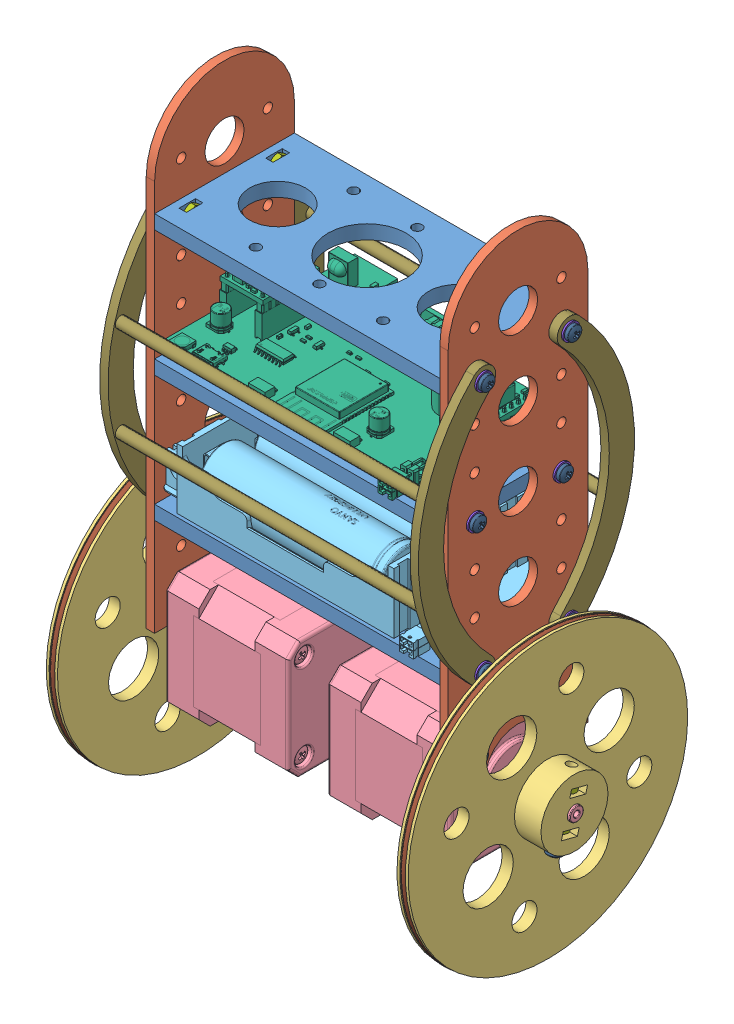
SolidWorks assembly RobotBalancin, configuration Predeterminado. Lengths in mm.
Overall size (150 233.71 126.43).
103 component instances, 13 part files, 199 mates.
Components (placement in the parent):
- RobotMiddle-1: RobotMiddle [Default] at (49.6239 154.592 64.1485) size (102 5 50)
- RobotLateral-1: RobotLateral [Default] at (100.3895 203.5472 64.288) size (3 165 50)
- RobotLateral-2: RobotLateral [Default] at (-4.6105 203.5472 64.288) size (3 165 50)
- RobotWheel-1: RobotWheel [Default] at (-11.3593 114.092 64.3829) x (0 -0.315254 -0.949007) z (-1 0 0) size (100 100 13.5)
- RobotWheel-2: RobotWheel [Default] at (110.074 114.092 64.3829) x (0 -0.248427 -0.968651) z (1 0 0) size (100 100 13.5)
- NEMA17-1: NEMA17 [Predeterminado] at (42.3895 109.4749 74.7784) x (0 0 1) z (-1 0 0) size (42.3 42.3 68)
- NEMA17-2: NEMA17 [Predeterminado] at (56.3895 109.4749 53.9874) x (0 0 -1) z (1 0 0) size (42.3 42.3 68)
- RobotMiddle-2: RobotMiddle [Default] at (49.6239 199.592 64.1485) size (102 5 50)
- RobotMiddle-3: RobotMiddle [Default] at (49.6239 244.592 64.1485) size (102 5 50)
- PowerBoard-4: PowerBoard [Predeterminado] at (99.6419 165.2035 39.6765) x (-1 0 0) z (0 1 0) size (100 62.58 25.48)
- ControlBoard-1: ControlBoard [Predeterminado] at (99.6279 210.2035 39.6365) x (-1 0 0) z (0 1 0) size (100 63.99 44.22)
- hex nut style 1 gradeab_iso-1: hex nut style 1 gradeab_iso [ISO - 4032 - M2.5 - D - N] at (97.0495 157.092 48.8829) x (0 0 -1) z (1 0 0) size (5 5.77 2)
- hex nut style 1 gradeab_iso-2: hex nut style 1 gradeab_iso [ISO - 4032 - M2.5 - D - N] at (1.6495 157.092 48.8829) x (0 0 1) z (-1 0 0) size (5 5.77 2)
- hex nut style 1 gradeab_iso-3: hex nut style 1 gradeab_iso [ISO - 4032 - M2.5 - D - N] at (1.6495 157.092 79.8829) x (0 0 1) z (-1 0 0) size (5 5.77 2)
- hex nut style 1 gradeab_iso-4: hex nut style 1 gradeab_iso [ISO - 4032 - M2.5 - D - N] at (97.0495 157.092 79.8829) x (0 0 -1) z (1 0 0) size (5 5.77 2)
- hex nut style 1 gradeab_iso-5: hex nut style 1 gradeab_iso [ISO - 4032 - M2.5 - D - N] at (97.0495 202.092 79.8829) x (0 0 -1) z (1 0 0) size (5 5.77 2)
- hex nut style 1 gradeab_iso-6: hex nut style 1 gradeab_iso [ISO - 4032 - M2.5 - D - N] at (97.0495 202.092 48.8829) x (0 0 -1) z (1 0 0) size (5 5.77 2)
- hex nut style 1 gradeab_iso-7: hex nut style 1 gradeab_iso [ISO - 4032 - M2.5 - D - N] at (1.6495 202.092 79.8829) x (0 0 1) z (-1 0 0) size (5 5.77 2)
- hex nut style 1 gradeab_iso-8: hex nut style 1 gradeab_iso [ISO - 4032 - M2.5 - D - N] at (1.6495 202.092 48.8829) x (0 0 1) z (-1 0 0) size (5 5.77 2)
- plain washer 10673 type snl_iso-1: plain washer 10673 type snl_iso [ISO 10673-2.75-S] at (49.6239 154.592 46.6485) x (0 -1 0) z (0 0 1) size (0.6 6 6)
- plain washer 10673 type snl_iso-2: plain washer 10673 type snl_iso [ISO 10673-2.75-S] at (72.3739 154.592 81.6485) x (0 -1 0) z (0 0 1) size (0.6 6 6)
- plain washer 10673 type snl_iso-3: plain washer 10673 type snl_iso [ISO 10673-2.75-S] at (26.8739 154.592 81.6485) x (0 -1 0) z (0 0 1) size (0.6 6 6)
- plain washer 10673 type snl_iso-6: plain washer 10673 type snl_iso [ISO 10673-2.75-S] at (-4.6105 202.092 79.8829) x (-1 0 0) z (0 0.924225 0.381849) size (0.6 6 6)
- plain washer 10673 type snl_iso-7: plain washer 10673 type snl_iso [ISO 10673-2.75-S] at (-4.6105 202.092 48.8829) x (-1 0 0) z (0 0.924225 0.381849) size (0.6 6 6)
- plain washer 10673 type snl_iso-12: plain washer 10673 type snl_iso [ISO 10673-2.75-S] at (103.3895 202.092 48.8829) size (0.6 6 6)
- plain washer 10673 type snl_iso-13: plain washer 10673 type snl_iso [ISO 10673-2.75-S] at (103.3895 202.092 79.8829) size (0.6 6 6)
- plain washer 10673 type snl_iso-17: plain washer 10673 type snl_iso [ISO 10673-2.75-S] at (72.3739 199.592 46.6485) x (0 -1 0) z (0 0 1) size (0.6 6 6)
- plain washer 10673 type snl_iso-18: plain washer 10673 type snl_iso [ISO 10673-2.75-S] at (26.8739 199.592 46.6485) x (0 -1 0) z (0 0 1) size (0.6 6 6)
- plain washer 10673 type snl_iso-19: plain washer 10673 type snl_iso [ISO 10673-2.75-S] at (49.6239 159.592 46.6485) x (0 1 0) z (0 0 1) size (0.6 6 6)
- plain washer 10673 type snl_iso-20: plain washer 10673 type snl_iso [ISO 10673-2.75-S] at (26.8739 159.592 81.6485) x (0 1 0) z (0 0 1) size (0.6 6 6)
- plain washer 10673 type snl_iso-21: plain washer 10673 type snl_iso [ISO 10673-2.75-S] at (72.3739 159.592 81.6485) x (0 1 0) z (0 0 1) size (0.6 6 6)
- plain washer 10673 type snl_iso-22: plain washer 10673 type snl_iso [ISO 10673-2.75-S] at (72.3739 204.592 46.6485) x (0 1 0) z (0 0 1) size (0.6 6 6)
- plain washer 10673 type snl_iso-23: plain washer 10673 type snl_iso [ISO 10673-2.75-S] at (26.8739 204.592 46.6485) x (0 1 0) z (0 0 1) size (0.6 6 6)
- hex nut style 1 gradeab_iso-9: hex nut style 1 gradeab_iso [ISO - 4032 - M2.5 - D - N] at (49.6239 162.192 46.6485) x (1 0 0) z (0 1 0) size (5 5.77 2)
- hex nut style 1 gradeab_iso-10: hex nut style 1 gradeab_iso [ISO - 4032 - M2.5 - D - N] at (72.3739 162.192 81.6485) x (1 0 0) z (0 1 0) size (5 5.77 2)
- hex nut style 1 gradeab_iso-11: hex nut style 1 gradeab_iso [ISO - 4032 - M2.5 - D - N] at (26.8739 162.192 81.6485) x (1 0 0) z (0 1 0) size (5 5.77 2)
- hex nut style 1 gradeab_iso-12: hex nut style 1 gradeab_iso [ISO - 4032 - M2.5 - D - N] at (26.8739 207.192 46.6485) x (1 0 0) z (0 1 0) size (5 5.77 2)
- hex nut style 1 gradeab_iso-15: hex nut style 1 gradeab_iso [ISO - 4032 - M2.5 - D - N] at (26.8739 209.192 46.6485) x (1 0 0) z (0 1 0) size (5 5.77 2)
- hex nut style 1 gradeab_iso-16: hex nut style 1 gradeab_iso [ISO - 4032 - M2.5 - D - N] at (26.8739 164.192 81.6485) x (1 0 0) z (0 1 0) size (5 5.77 2)
- hex nut style 1 gradeab_iso-17: hex nut style 1 gradeab_iso [ISO - 4032 - M2.5 - D - N] at (49.6239 164.192 46.6485) x (1 0 0) z (0 1 0) size (5 5.77 2)
- hex nut style 1 gradeab_iso-18: hex nut style 1 gradeab_iso [ISO - 4032 - M2.5 - D - N] at (72.3739 164.192 81.6485) x (1 0 0) z (0 1 0) size (5 5.77 2)
- hex nut style 1 gradeab_iso-20: hex nut style 1 gradeab_iso [ISO - 4032 - M2.5 - D - N] at (72.3739 207.192 46.6485) x (1 0 0) z (0 1 0) size (5 5.77 2)
- hex nut style 1 gradeab_iso-21: hex nut style 1 gradeab_iso [ISO - 4032 - M2.5 - D - N] at (72.3739 209.192 46.6485) x (1 0 0) z (0 1 0) size (5 5.77 2)
- plain washer 10673 type snl_iso-24: plain washer 10673 type snl_iso [ISO 10673-2.75-S] at (72.3739 209.192 46.6485) x (0 1 0) z (0 0 1) size (0.6 6 6)
- plain washer 10673 type snl_iso-25: plain washer 10673 type snl_iso [ISO 10673-2.75-S] at (26.8739 209.192 46.6485) x (0 1 0) z (0 0 1) size (0.6 6 6)
- plain washer 10673 type snl_iso-26: plain washer 10673 type snl_iso [ISO 10673-2.75-S] at (26.8739 164.192 81.6485) x (0 1 0) z (0 0 1) size (0.6 6 6)
- plain washer 10673 type snl_iso-27: plain washer 10673 type snl_iso [ISO 10673-2.75-S] at (72.3739 164.192 81.6485) x (0 1 0) z (0 0 1) size (0.6 6 6)
- plain washer 10673 type snl_iso-28: plain washer 10673 type snl_iso [ISO 10673-2.75-S] at (49.6239 164.192 46.6485) x (0 1 0) z (0 0 1) size (0.6 6 6)
- plain washer 10673 type snl_iso-30: plain washer 10673 type snl_iso [ISO 10673-2.75-S] at (72.3739 210.2035 46.6485) x (0 1 0) z (0 0 1) size (0.6 6 6)
- plain washer 10673 type snl_iso-31: plain washer 10673 type snl_iso [ISO 10673-2.75-S] at (26.8739 210.2035 46.6485) x (0 1 0) z (0 0 1) size (0.6 6 6)
- countersunk flat head cross recess screw_iso-1: countersunk flat head cross recess screw_iso [ISO 7046-1 - M2.5 x 16 - Z - 16N] at (49.6155 166.8314 46.6547) x (0 -1 0) z (0.014601 0 0.999893) size (16 4.7 4.7)
- countersunk flat head cross recess screw_iso-2: countersunk flat head cross recess screw_iso [ISO 7046-1 - M2.5 x 16 - Z - 16N] at (72.3655 166.8314 81.6547) x (0 -1 0) z (-0.020315 0 0.999794) size (16 4.7 4.7)
- countersunk flat head cross recess screw_iso-3: countersunk flat head cross recess screw_iso [ISO 7046-1 - M2.5 x 16 - Z - 16N] at (26.8655 166.8314 81.6547) x (0 -1 0) z (-0.013089 0 0.999914) size (16 4.7 4.7)
- pan head cross recess screw_iso-1: pan head cross recess screw_iso [ISO 7045 - M2.5 x 16 - Z - 16N] at (72.3739 212.9035 46.6485) x (0 -1 0) z (0 0 1) size (18.05 5 5)
- pan head cross recess screw_iso-2: pan head cross recess screw_iso [ISO 7045 - M2.5 x 16 - Z - 16N] at (26.8739 212.9035 46.6485) x (0 -1 0) z (0 0 1) size (18.05 5 5)
- pan head cross recess screw_iso-5: pan head cross recess screw_iso [ISO 7045 - M2.5 x 8 - Z - 8N] at (106.0895 202.092 48.8829) x (-1 0 0) z (0 0.924225 0.381849) size (10.05 5 5)
- pan head cross recess screw_iso-6: pan head cross recess screw_iso [ISO 7045 - M2.5 x 8 - Z - 8N] at (106.0895 202.092 79.8829) x (-1 0 0) z (0 0.924225 0.381849) size (10.05 5 5)
- pan head cross recess screw_iso-11: pan head cross recess screw_iso [ISO 7045 - M2.5 x 8 - Z - 8N] at (-7.3105 202.092 79.8829) size (10.05 5 5)
- pan head cross recess screw_iso-12: pan head cross recess screw_iso [ISO 7045 - M2.5 x 8 - Z - 8N] at (-7.3105 202.092 48.8829) size (10.05 5 5)
- plain washer 10673 type snl_iso-32: plain washer 10673 type snl_iso [ISO 10673-2.75-S] at (103.3895 129.592 48.8829) size (0.6 6 6)
- plain washer 10673 type snl_iso-33: plain washer 10673 type snl_iso [ISO 10673-2.75-S] at (103.3895 129.592 79.8829) size (0.6 6 6)
- plain washer 10673 type snl_iso-34: plain washer 10673 type snl_iso [ISO 10673-2.75-S] at (-4.6105 129.592 48.8829) x (-1 0 0) z (0 0.924225 0.381849) size (0.6 6 6)
- plain washer 10673 type snl_iso-35: plain washer 10673 type snl_iso [ISO 10673-2.75-S] at (-4.6105 129.592 79.8829) x (-1 0 0) z (0 0.924225 0.381849) size (0.6 6 6)
- pan head cross recess screw_iso-17: pan head cross recess screw_iso [ISO 7045 - M3 x 8 - Z - 8N] at (-7.6105 129.592 48.8829) size (10.35 5.6 5.6)
- pan head cross recess screw_iso-18: pan head cross recess screw_iso [ISO 7045 - M3 x 8 - Z - 8N] at (-7.6105 129.592 79.8829) size (10.35 5.6 5.6)
- pan head cross recess screw_iso-19: pan head cross recess screw_iso [ISO 7045 - M3 x 8 - Z - 8N] at (106.3895 129.592 48.8829) x (-1 0 0) z (0 0.924225 0.381849) size (10.35 5.6 5.6)
- pan head cross recess screw_iso-20: pan head cross recess screw_iso [ISO 7045 - M3 x 8 - Z - 8N] at (106.3895 129.592 79.8829) x (-1 0 0) z (0 0.924225 0.381849) size (10.35 5.6 5.6)
- hex nut style 1 gradeab_iso-22: hex nut style 1 gradeab_iso [ISO - 4032 - M2.5 - D - N] at (119.574 120.582 62.7184) x (1 0 0) z (0 0.968651 -0.248427) size (5 5.77 2)
- hex nut style 1 gradeab_iso-23: hex nut style 1 gradeab_iso [ISO - 4032 - M2.5 - D - N] at (119.574 107.6021 66.0474) x (1 0 0) z (0 -0.968651 0.248427) size (5 5.77 2)
- hex nut style 1 gradeab_iso-24: hex nut style 1 gradeab_iso [ISO - 4032 - M2.5 - D - N] at (-20.8593 120.4504 62.2707) x (1 0 0) z (0 0.949007 -0.315254) size (5 5.77 2)
- hex nut style 1 gradeab_iso-25: hex nut style 1 gradeab_iso [ISO - 4032 - M2.5 - D - N] at (-20.8593 107.7337 66.4951) x (1 0 0) z (0 -0.949007 0.315254) size (5 5.77 2)
- pan head cross recess screw_iso-23: pan head cross recess screw_iso [ISO 7045 - M2.5 x 20 - Z - 20N] at (-20.8593 127.473 59.9378) x (0 -0.949007 0.315254) z (-0.315254 0.299178 0.900615) size (22.05 5 5)
- pan head cross recess screw_iso-24: pan head cross recess screw_iso [ISO 7045 - M2.5 x 20 - Z - 20N] at (119.574 100.4341 67.8857) x (0 0.968651 -0.248427) z (0.248427 0.240639 0.938284) size (22.05 5 5)
- o-rings series g_iso-1: o-rings series g_iso [O-ring 95x2.65-B-ISO 3601-1] at (-13.3052 114.092 64.3829) x (0 0 1) z (-1 0 0) size (100.3 100.3 2.65)
- o-rings series g_iso-2: o-rings series g_iso [O-ring 95x2.65-B-ISO 3601-1] at (112.1974 114.092 64.3829) x (0 0 -1) z (1 0 0) size (100.3 100.3 2.65)
- hex nut style 1 gradeab_iso-27: hex nut style 1 gradeab_iso [ISO - 4032 - M2.5 - D - N] at (97.0495 247.092 48.8829) x (0 0 -1) z (1 0 0) size (5 5.77 2)
- hex nut style 1 gradeab_iso-28: hex nut style 1 gradeab_iso [ISO - 4032 - M2.5 - D - N] at (97.0495 247.092 79.8829) x (0 0 -1) z (1 0 0) size (5 5.77 2)
- hex nut style 1 gradeab_iso-29: hex nut style 1 gradeab_iso [ISO - 4032 - M2.5 - D - N] at (1.6495 247.092 48.8829) x (0 0 1) z (-1 0 0) size (5 5.77 2)
- hex nut style 1 gradeab_iso-30: hex nut style 1 gradeab_iso [ISO - 4032 - M2.5 - D - N] at (1.6495 247.092 79.8829) x (0 0 1) z (-1 0 0) size (5 5.77 2)
- plain washer 10673 type snl_iso-40: plain washer 10673 type snl_iso [ISO 10673-2.75-S] at (-7.6105 157.092 48.8829) x (-1 0 0) z (0 0.924225 0.381849) size (0.6 6 6)
- plain washer 10673 type snl_iso-41: plain washer 10673 type snl_iso [ISO 10673-2.75-S] at (-7.6105 247.0945 48.8829) x (-1 0 0) z (0 0.924225 0.381849) size (0.6 6 6)
- plain washer 10673 type snl_iso-42: plain washer 10673 type snl_iso [ISO 10673-2.75-S] at (-7.6105 247.0945 79.8829) x (-1 0 0) z (0 0.924225 0.381849) size (0.6 6 6)
- plain washer 10673 type snl_iso-43: plain washer 10673 type snl_iso [ISO 10673-2.75-S] at (-7.6105 157.092 79.8829) x (-1 0 0) z (0 0.924225 0.381849) size (0.6 6 6)
- plain washer 10673 type snl_iso-44: plain washer 10673 type snl_iso [ISO 10673-2.75-S] at (106.3895 247.0945 48.8829) size (0.6 6 6)
- plain washer 10673 type snl_iso-45: plain washer 10673 type snl_iso [ISO 10673-2.75-S] at (106.3895 247.0945 79.8829) size (0.6 6 6)
- plain washer 10673 type snl_iso-46: plain washer 10673 type snl_iso [ISO 10673-2.75-S] at (106.2803 157.2246 48.9253) size (0.6 6 6)
- plain washer 10673 type snl_iso-47: plain washer 10673 type snl_iso [ISO 10673-2.75-S] at (106.3895 157.092 79.8829) size (0.6 6 6)
- pan head cross recess screw_iso-32: pan head cross recess screw_iso [ISO 7045 - M2.5 x 10 - Z - 10N] at (109.0895 247.0945 79.8829) x (-1 0 0) z (0 0.924225 0.381849) size (12.05 5 5)
- pan head cross recess screw_iso-33: pan head cross recess screw_iso [ISO 7045 - M2.5 x 10 - Z - 10N] at (109.0895 247.0945 48.8829) x (-1 0 0) z (0 0.924225 0.381849) size (12.05 5 5)
- pan head cross recess screw_iso-34: pan head cross recess screw_iso [ISO 7045 - M2.5 x 10 - Z - 10N] at (108.9803 157.2246 48.9253) x (-1 0 0) z (0 0.924225 0.381849) size (12.05 5 5)
- pan head cross recess screw_iso-35: pan head cross recess screw_iso [ISO 7045 - M2.5 x 10 - Z - 10N] at (109.0895 157.092 79.8829) x (-1 0 0) z (0 0.924225 0.381849) size (12.05 5 5)
- pan head cross recess screw_iso-36: pan head cross recess screw_iso [ISO 7045 - M2.5 x 10 - Z - 10N] at (-10.3105 247.0945 48.8829) size (12.05 5 5)
- pan head cross recess screw_iso-37: pan head cross recess screw_iso [ISO 7045 - M2.5 x 10 - Z - 10N] at (-10.3105 247.0945 79.8829) size (12.05 5 5)
- pan head cross recess screw_iso-38: pan head cross recess screw_iso [ISO 7045 - M2.5 x 10 - Z - 10N] at (-10.3105 157.092 48.8829) size (12.05 5 5)
- pan head cross recess screw_iso-39: pan head cross recess screw_iso [ISO 7045 - M2.5 x 10 - Z - 10N] at (-10.3105 157.092 79.8829) size (12.05 5 5)
- hex nut style 1 gradeab_iso-32: hex nut style 1 gradeab_iso [ISO - 4032 - M2.5 - D - N] at (72.3739 196.992 46.6485) x (1 0 0) z (0 -1 0) size (5 5.77 2)
- hex nut style 1 gradeab_iso-33: hex nut style 1 gradeab_iso [ISO - 4032 - M2.5 - D - N] at (26.8739 196.992 46.6485) x (1 0 0) z (0 -1 0) size (5 5.77 2)
- hex nut style 1 gradeab_iso-34: hex nut style 1 gradeab_iso [ISO - 4032 - M2.5 - D - N] at (72.3739 151.992 81.6485) x (1 0 0) z (0 -1 0) size (5 5.77 2)
- hex nut style 1 gradeab_iso-35: hex nut style 1 gradeab_iso [ISO - 4032 - M2.5 - D - N] at (49.6239 151.992 46.6485) x (1 0 0) z (0 -1 0) size (5 5.77 2)
- hex nut style 1 gradeab_iso-36: hex nut style 1 gradeab_iso [ISO - 4032 - M2.5 - D - N] at (26.8739 151.992 81.6485) x (1 0 0) z (0 -1 0) size (5 5.77 2)
- protector-4: protector [Default] at (103.3895 200.9738 36.429) size (114 99 27.66)
- protector-5: protector [Default] at (-4.6105 200.9738 92.3367) x (-1 0 0) z (0 0 -1) size (114 99 27.66)
- PCBSupport-2: PCBSupport [Default] at (49.6239 199.592 81.6485) size (48.94 10.2 3.48)
Mates (geometry in assembly coordinates):
- Coincident2: coincident anti-aligned: circle of RobotMiddle-1; circle of RobotLateral-2
- Coincident4: coincident anti-aligned: circle of RobotMiddle-1; circle of RobotLateral-2
- Coincident5: coincident aligned: circle of RobotMiddle-1; circle of RobotLateral-1
- Coincident7: coincident aligned: circle of RobotMiddle-1; circle of RobotLateral-1
- Concentric1: concentric anti-aligned: circle of RobotLateral-1; circle of NEMA17-2
- Concentric2: concentric anti-aligned: circle of RobotLateral-1; circle of NEMA17-2
- Coincident8: coincident anti-aligned: plane of RobotLateral-1 through (100.3895 259.592 64.3829) normal (-1 0 0); plane of NEMA17-2 through (100.3895 114.092 64.3829) normal (1 0 0)
- Concentric3: concentric aligned: circle of RobotLateral-2; circle of NEMA17-1
- Concentric4: concentric aligned: circle of RobotLateral-2; circle of NEMA17-1
- Coincident9: coincident anti-aligned: plane of RobotLateral-2 through (-1.6105 259.592 64.3829) normal (1 0 0); plane of NEMA17-1 through (-1.6105 114.092 64.3829) normal (-1 0 0)
- Concentric5: concentric anti-aligned: cylinder of RobotWheel-1 through (11.1407 114.092 64.3829) axis (-1 0 0) radius 2.55; cylinder of NEMA17-1 through (-25.6105 114.092 64.3829) axis (1 0 0) radius 2.5
- Concentric6: concentric anti-aligned: cylinder of RobotWheel-2 through (87.574 114.092 64.3829) axis (1 0 0) radius 2.55; cylinder of NEMA17-2 through (124.3895 114.092 64.3829) axis (-1 0 0) radius 2.5
- Coincident10: coincident aligned: circle of RobotLateral-1; circle of RobotMiddle-2
- Coincident11: coincident aligned: circle of RobotLateral-1; circle of RobotMiddle-3
- Coincident12: coincident anti-aligned: circle of RobotLateral-2; circle of RobotMiddle-2
- Coincident13: coincident anti-aligned: circle of RobotLateral-2; circle of RobotMiddle-3
- Concentric7: concentric aligned: cylinder of RobotMiddle-1 through (80.3895 157.092 48.8829) axis (1 0 0) radius 1.68; cylinder of hex nut style 1 gradeab_iso-1 through (72.012 157.092 48.8829) axis (1 0 0) radius 1.25
- Coincident20: coincident anti-aligned: plane of RobotMiddle-1 through (95.0495 159.592 46.3829) normal (1 0 0); plane of hex nut style 1 gradeab_iso-1 through (95.0495 159.9788 48.8829) normal (-1 0 0)
- Concentric8: concentric aligned: cylinder of RobotMiddle-1 through (18.3895 157.092 48.8829) axis (-1 0 0) radius 1.68; cylinder of hex nut style 1 gradeab_iso-2 through (26.687 157.092 48.8829) axis (-1 0 0) radius 1.25
- Coincident21: coincident anti-aligned: plane of RobotMiddle-1 through (3.6495 159.592 46.3829) normal (-1 0 0); plane of hex nut style 1 gradeab_iso-2 through (3.6495 159.9788 48.8829) normal (1 0 0)
- Concentric9: concentric aligned: cylinder of RobotMiddle-1 through (18.3895 157.092 79.8829) axis (-1 0 0) radius 1.68; cylinder of hex nut style 1 gradeab_iso-3 through (26.687 157.092 79.8829) axis (-1 0 0) radius 1.25
- Coincident22: coincident anti-aligned: plane of RobotMiddle-1 through (3.6495 159.592 77.3829) normal (-1 0 0); plane of hex nut style 1 gradeab_iso-3 through (3.6495 159.9788 79.8829) normal (1 0 0)
- Concentric10: concentric aligned: cylinder of RobotMiddle-1 through (80.3895 157.092 79.8829) axis (1 0 0) radius 1.68; cylinder of hex nut style 1 gradeab_iso-4 through (72.012 157.092 79.8829) axis (1 0 0) radius 1.25
- Coincident23: coincident anti-aligned: plane of RobotMiddle-1 through (95.0495 159.592 77.3829) normal (1 0 0); plane of hex nut style 1 gradeab_iso-4 through (95.0495 159.9788 79.8829) normal (-1 0 0)
- Concentric11: concentric aligned: cylinder of RobotMiddle-2 through (80.3895 202.092 79.8829) axis (1 0 0) radius 1.68; cylinder of hex nut style 1 gradeab_iso-5 through (72.012 202.092 79.8829) axis (1 0 0) radius 1.25
- Coincident24: coincident anti-aligned: plane of RobotMiddle-2 through (95.0495 204.592 77.3829) normal (1 0 0); plane of hex nut style 1 gradeab_iso-5 through (95.0495 204.9788 79.8829) normal (-1 0 0)
- Concentric12: concentric aligned: cylinder of RobotMiddle-2 through (80.3895 202.092 48.8829) axis (1 0 0) radius 1.68; cylinder of hex nut style 1 gradeab_iso-6 through (72.012 202.092 48.8829) axis (1 0 0) radius 1.25
- Coincident25: coincident anti-aligned: plane of RobotMiddle-2 through (95.0495 204.592 46.3829) normal (1 0 0); plane of hex nut style 1 gradeab_iso-6 through (95.0495 204.9788 48.8829) normal (-1 0 0)
- Concentric13: concentric aligned: cylinder of RobotMiddle-2 through (18.3895 202.092 79.8829) axis (-1 0 0) radius 1.68; cylinder of hex nut style 1 gradeab_iso-7 through (26.687 202.092 79.8829) axis (-1 0 0) radius 1.25
- Coincident26: coincident anti-aligned: plane of RobotMiddle-2 through (3.6495 204.592 77.3829) normal (-1 0 0); plane of hex nut style 1 gradeab_iso-7 through (3.6495 204.9788 79.8829) normal (1 0 0)
- Concentric14: concentric aligned: cylinder of RobotMiddle-2 through (18.3895 202.092 48.8829) axis (-1 0 0) radius 1.68; cylinder of hex nut style 1 gradeab_iso-8 through (26.687 202.092 48.8829) axis (-1 0 0) radius 1.25
- Coincident27: coincident anti-aligned: plane of RobotMiddle-2 through (3.6495 204.592 46.3829) normal (-1 0 0); plane of hex nut style 1 gradeab_iso-8 through (3.6495 204.9788 48.8829) normal (1 0 0)
- Concentric15: concentric aligned: cylinder of RobotMiddle-1 through (49.6239 154.592 46.6485) axis (0 1 0) radius 1.72; cylinder of plain washer 10673 type snl_iso-1 through (49.6239 153.992 46.6485) axis (0 1 0) radius 1.375
- Coincident32: coincident anti-aligned: plane of RobotMiddle-1 through (49.6239 154.592 64.1485) normal (0 -1 0); plane of plain washer 10673 type snl_iso-1 through (49.6239 154.592 46.6485) normal (0 1 0)
- Concentric16: concentric aligned: cylinder of RobotMiddle-1 through (72.3739 154.592 81.6485) axis (0 1 0) radius 1.72; cylinder of plain washer 10673 type snl_iso-2 through (72.3739 153.992 81.6485) axis (0 1 0) radius 1.375
- Coincident33: coincident anti-aligned: plane of RobotMiddle-1 through (49.6239 154.592 64.1485) normal (0 -1 0); plane of plain washer 10673 type snl_iso-2 through (72.3739 154.592 81.6485) normal (0 1 0)
- Concentric17: concentric aligned: cylinder of RobotMiddle-1 through (26.8739 154.592 81.6485) axis (0 1 0) radius 1.72; cylinder of plain washer 10673 type snl_iso-3 through (26.8739 153.992 81.6485) axis (0 1 0) radius 1.375
- Coincident34: coincident anti-aligned: plane of RobotMiddle-1 through (49.6239 154.592 64.1485) normal (0 -1 0); plane of plain washer 10673 type snl_iso-3 through (26.8739 154.592 81.6485) normal (0 1 0)
- Concentric20: concentric aligned: cylinder of RobotLateral-2 through (-4.6105 202.092 79.8829) axis (1 0 0) radius 1.68; cylinder of plain washer 10673 type snl_iso-6 through (-5.2105 202.092 79.8829) axis (1 0 0) radius 1.375
- Coincident36: coincident anti-aligned: plane of RobotLateral-2 through (-4.6105 259.592 64.3829) normal (-1 0 0); plane of plain washer 10673 type snl_iso-6 through (-4.6105 202.092 79.8829) normal (1 0 0)
- Concentric21: concentric aligned: cylinder of RobotLateral-2 through (-4.6105 202.092 48.8829) axis (1 0 0) radius 1.68; cylinder of plain washer 10673 type snl_iso-7 through (-5.2105 202.092 48.8829) axis (1 0 0) radius 1.375
- Coincident37: coincident anti-aligned: plane of RobotLateral-2 through (-4.6105 259.592 64.3829) normal (-1 0 0); plane of plain washer 10673 type snl_iso-7 through (-4.6105 202.092 48.8829) normal (1 0 0)
- Concentric26: concentric anti-aligned: cylinder of RobotLateral-1 through (100.3895 202.092 48.8829) axis (1 0 0) radius 1.68; cylinder of plain washer 10673 type snl_iso-12 through (103.9895 202.092 48.8829) axis (-1 0 0) radius 1.375
- Coincident42: coincident anti-aligned: plane of RobotLateral-1 through (103.3895 259.592 64.3829) normal (1 0 0); plane of plain washer 10673 type snl_iso-12 through (103.3895 202.092 48.8829) normal (-1 0 0)
- Concentric27: concentric anti-aligned: cylinder of RobotLateral-1 through (100.3895 202.092 79.8829) axis (1 0 0) radius 1.68; cylinder of plain washer 10673 type snl_iso-13 through (103.9895 202.092 79.8829) axis (-1 0 0) radius 1.375
- Coincident43: coincident anti-aligned: plane of RobotLateral-1 through (103.3895 259.592 64.3829) normal (1 0 0); plane of plain washer 10673 type snl_iso-13 through (103.3895 202.092 79.8829) normal (-1 0 0)
- Concentric311: concentric aligned: cylinder of RobotMiddle-2 through (72.3739 199.592 46.6485) axis (0 1 0) radius 1.72; cylinder of plain washer 10673 type snl_iso-17 through (72.3739 198.992 46.6485) axis (0 1 0) radius 1.375
- Coincident461: coincident anti-aligned: plane of RobotMiddle-2 through (49.6239 199.592 64.1485) normal (0 -1 0); plane of plain washer 10673 type snl_iso-17 through (72.3739 199.592 46.6485) normal (0 1 0)
- Concentric32: concentric aligned: cylinder of RobotMiddle-2 through (26.8739 199.592 46.6485) axis (0 1 0) radius 1.72; cylinder of plain washer 10673 type snl_iso-18 through (26.8739 198.992 46.6485) axis (0 1 0) radius 1.375
- Coincident47: coincident anti-aligned: plane of RobotMiddle-2 through (49.6239 199.592 64.1485) normal (0 -1 0); plane of plain washer 10673 type snl_iso-18 through (26.8739 199.592 46.6485) normal (0 1 0)
- Concentric33: concentric anti-aligned: cylinder of RobotMiddle-1 through (49.6239 154.592 46.6485) axis (0 1 0) radius 1.72; cylinder of plain washer 10673 type snl_iso-19 through (49.6239 160.192 46.6485) axis (0 -1 0) radius 1.375
- Coincident48: coincident anti-aligned: plane of RobotMiddle-1 through (49.6239 159.592 64.1485) normal (0 1 0); plane of plain washer 10673 type snl_iso-19 through (49.6239 159.592 46.6485) normal (0 -1 0)
- Concentric34: concentric anti-aligned: cylinder of RobotMiddle-1 through (26.8739 154.592 81.6485) axis (0 1 0) radius 1.72; cylinder of plain washer 10673 type snl_iso-20 through (26.8739 160.192 81.6485) axis (0 -1 0) radius 1.375
- Coincident49: coincident anti-aligned: plane of RobotMiddle-1 through (49.6239 159.592 64.1485) normal (0 1 0); plane of plain washer 10673 type snl_iso-20 through (26.8739 159.592 81.6485) normal (0 -1 0)
- Concentric35: concentric anti-aligned: cylinder of RobotMiddle-1 through (72.3739 154.592 81.6485) axis (0 1 0) radius 1.72; cylinder of plain washer 10673 type snl_iso-21 through (72.3739 160.192 81.6485) axis (0 -1 0) radius 1.375
- Coincident50: coincident anti-aligned: plane of RobotMiddle-1 through (49.6239 159.592 64.1485) normal (0 1 0); plane of plain washer 10673 type snl_iso-21 through (72.3739 159.592 81.6485) normal (0 -1 0)
- Concentric36: concentric anti-aligned: cylinder of RobotMiddle-2 through (72.3739 199.592 46.6485) axis (0 1 0) radius 1.72; cylinder of plain washer 10673 type snl_iso-22 through (72.3739 205.192 46.6485) axis (0 -1 0) radius 1.375
- Coincident51: coincident anti-aligned: plane of RobotMiddle-2 through (49.6239 204.592 64.1485) normal (0 1 0); plane of plain washer 10673 type snl_iso-22 through (72.3739 204.592 46.6485) normal (0 -1 0)
- Concentric37: concentric anti-aligned: cylinder of RobotMiddle-2 through (26.8739 199.592 46.6485) axis (0 1 0) radius 1.72; cylinder of plain washer 10673 type snl_iso-23 through (26.8739 205.192 46.6485) axis (0 -1 0) radius 1.375
- Coincident52: coincident anti-aligned: plane of RobotMiddle-2 through (49.6239 204.592 64.1485) normal (0 1 0); plane of plain washer 10673 type snl_iso-23 through (26.8739 204.592 46.6485) normal (0 -1 0)
- Concentric38: concentric anti-aligned: cylinder of plain washer 10673 type snl_iso-19 through (49.6239 160.192 46.6485) axis (0 -1 0) radius 3; cylinder of hex nut style 1 gradeab_iso-9 through (49.6239 137.1545 46.6485) axis (0 1 0) radius 1.25
- Coincident53: coincident anti-aligned: plane of plain washer 10673 type snl_iso-19 through (49.6239 160.192 46.6485) normal (0 1 0); plane of hex nut style 1 gradeab_iso-9 through (49.6239 160.192 43.7618) normal (0 -1 0)
- Concentric39: concentric anti-aligned: cylinder of plain washer 10673 type snl_iso-21 through (72.3739 160.192 81.6485) axis (0 -1 0) radius 1.375; cylinder of hex nut style 1 gradeab_iso-10 through (72.3739 137.1545 81.6485) axis (0 1 0) radius 1.25
- Coincident54: coincident anti-aligned: plane of plain washer 10673 type snl_iso-21 through (72.3739 160.192 81.6485) normal (0 1 0); plane of hex nut style 1 gradeab_iso-10 through (72.3739 160.192 78.7618) normal (0 -1 0)
- Concentric40: concentric anti-aligned: cylinder of plain washer 10673 type snl_iso-20 through (26.8739 160.192 81.6485) axis (0 -1 0) radius 3; cylinder of hex nut style 1 gradeab_iso-11 through (26.8739 137.1545 81.6485) axis (0 1 0) radius 1.25
- Coincident55: coincident anti-aligned: plane of plain washer 10673 type snl_iso-20 through (26.8739 160.192 81.6485) normal (0 1 0); plane of hex nut style 1 gradeab_iso-11 through (26.8739 160.192 78.7618) normal (0 -1 0)
- Concentric41: concentric anti-aligned: cylinder of plain washer 10673 type snl_iso-23 through (26.8739 205.192 46.6485) axis (0 -1 0) radius 3; cylinder of hex nut style 1 gradeab_iso-12 through (26.8739 182.1545 46.6485) axis (0 1 0) radius 1.25
- Coincident56: coincident anti-aligned: plane of plain washer 10673 type snl_iso-23 through (26.8739 205.192 46.6485) normal (0 1 0); plane of hex nut style 1 gradeab_iso-12 through (26.8739 205.192 43.7618) normal (0 -1 0)
- Concentric44: concentric anti-aligned: cone of hex nut style 1 gradeab_iso-12 through (26.8739 207.0187 46.6485) axis (0 -1 0); cylinder of hex nut style 1 gradeab_iso-15 through (26.8739 184.1545 46.6485) axis (0 1 0) radius 1.25
- Coincident59: coincident anti-aligned: plane of hex nut style 1 gradeab_iso-12 through (26.8739 207.192 43.7618) normal (0 1 0); plane of hex nut style 1 gradeab_iso-15 through (26.8739 207.192 43.7618) normal (0 -1 0)
- Concentric45: concentric aligned: cone of hex nut style 1 gradeab_iso-11 through (26.8739 162.192 81.6485) axis (0 1 0); cylinder of hex nut style 1 gradeab_iso-16 through (26.8739 139.1545 81.6485) axis (0 1 0) radius 1.25
- Coincident60: coincident anti-aligned: plane of hex nut style 1 gradeab_iso-11 through (26.8739 162.192 78.7618) normal (0 1 0); plane of hex nut style 1 gradeab_iso-16 through (26.8739 162.192 78.7618) normal (0 -1 0)
- Concentric46: concentric aligned: cone of hex nut style 1 gradeab_iso-9 through (49.6239 162.192 46.6485) axis (0 1 0); cylinder of hex nut style 1 gradeab_iso-17 through (49.6239 139.1545 46.6485) axis (0 1 0) radius 1.25
- Coincident61: coincident anti-aligned: plane of hex nut style 1 gradeab_iso-9 through (49.6239 162.192 43.7618) normal (0 1 0); plane of hex nut style 1 gradeab_iso-17 through (49.6239 162.192 43.7618) normal (0 -1 0)
- Concentric47: concentric anti-aligned: cone of hex nut style 1 gradeab_iso-10 through (72.3739 162.0187 81.6485) axis (0 -1 0); cylinder of hex nut style 1 gradeab_iso-18 through (72.3739 139.1545 81.6485) axis (0 1 0) radius 1.25
- Coincident62: coincident anti-aligned: plane of hex nut style 1 gradeab_iso-10 through (72.3739 162.192 78.7618) normal (0 1 0); plane of hex nut style 1 gradeab_iso-18 through (72.3739 162.192 78.7618) normal (0 -1 0)
- Concentric49: concentric anti-aligned: cylinder of plain washer 10673 type snl_iso-22 through (72.3739 205.192 46.6485) axis (0 -1 0) radius 3; cylinder of hex nut style 1 gradeab_iso-20 through (72.3739 182.1545 46.6485) axis (0 1 0) radius 1.25
- Coincident64: coincident anti-aligned: plane of plain washer 10673 type snl_iso-22 through (72.3739 205.192 46.6485) normal (0 1 0); plane of hex nut style 1 gradeab_iso-20 through (72.3739 205.192 43.7618) normal (0 -1 0)
- Concentric50: concentric anti-aligned: cone of hex nut style 1 gradeab_iso-20 through (72.3739 207.0187 46.6485) axis (0 -1 0); cylinder of hex nut style 1 gradeab_iso-21 through (72.3739 184.1545 46.6485) axis (0 1 0) radius 1.25
- Coincident65: coincident anti-aligned: plane of hex nut style 1 gradeab_iso-20 through (72.3739 207.192 43.7618) normal (0 1 0); plane of hex nut style 1 gradeab_iso-21 through (72.3739 207.192 43.7618) normal (0 -1 0)
- Concentric51: concentric aligned: cone of hex nut style 1 gradeab_iso-21 through (72.3739 209.0187 46.6485) axis (0 -1 0); cylinder of plain washer 10673 type snl_iso-24 through (72.3739 209.792 46.6485) axis (0 -1 0) radius 1.375
- Coincident66: coincident anti-aligned: plane of hex nut style 1 gradeab_iso-21 through (72.3739 209.192 43.7618) normal (0 1 0); plane of plain washer 10673 type snl_iso-24 through (72.3739 209.192 46.6485) normal (0 -1 0)
- Concentric52: concentric aligned: cone of hex nut style 1 gradeab_iso-15 through (26.8739 209.0187 46.6485) axis (0 -1 0); cylinder of plain washer 10673 type snl_iso-25 through (26.8739 209.792 46.6485) axis (0 -1 0) radius 1.375
- Coincident67: coincident anti-aligned: plane of hex nut style 1 gradeab_iso-15 through (26.8739 209.192 43.7618) normal (0 1 0); plane of plain washer 10673 type snl_iso-25 through (26.8739 209.192 46.6485) normal (0 -1 0)
- Concentric53: concentric anti-aligned: cone of hex nut style 1 gradeab_iso-16 through (26.8739 164.192 81.6485) axis (0 1 0); cylinder of plain washer 10673 type snl_iso-26 through (26.8739 164.792 81.6485) axis (0 -1 0) radius 1.375
- Coincident68: coincident anti-aligned: plane of hex nut style 1 gradeab_iso-16 through (26.8739 164.192 78.7618) normal (0 1 0); plane of plain washer 10673 type snl_iso-26 through (26.8739 164.192 81.6485) normal (0 -1 0)
- Concentric54: concentric anti-aligned: cone of hex nut style 1 gradeab_iso-18 through (72.3739 164.192 81.6485) axis (0 1 0); cylinder of plain washer 10673 type snl_iso-27 through (72.3739 164.792 81.6485) axis (0 -1 0) radius 1.375
- Coincident69: coincident anti-aligned: plane of hex nut style 1 gradeab_iso-18 through (72.3739 164.192 78.7618) normal (0 1 0); plane of plain washer 10673 type snl_iso-27 through (72.3739 164.192 81.6485) normal (0 -1 0)
- Concentric55: concentric aligned: cone of hex nut style 1 gradeab_iso-17 through (49.6239 164.0187 46.6485) axis (0 -1 0); cylinder of plain washer 10673 type snl_iso-28 through (49.6239 164.792 46.6485) axis (0 -1 0) radius 1.375
- Coincident70: coincident anti-aligned: plane of hex nut style 1 gradeab_iso-17 through (49.6239 164.192 43.7618) normal (0 1 0); plane of plain washer 10673 type snl_iso-28 through (49.6239 164.192 46.6485) normal (0 -1 0)
- Concentric56: concentric aligned: circle of PowerBoard-4; circle of plain washer 10673 type snl_iso-28
- Concentric57: concentric aligned: circle of PowerBoard-4; circle of plain washer 10673 type snl_iso-27
- Coincident71: coincident anti-aligned: plane of PowerBoard-4 through (-0.3961 164.792 42.1485) normal (0 -1 0); plane of plain washer 10673 type snl_iso-28 through (49.6239 164.792 46.6485) normal (0 1 0)
- Concentric59: concentric aligned: circle of ControlBoard-1; circle of plain washer 10673 type snl_iso-25
- Concentric60: concentric aligned: circle of ControlBoard-1; circle of plain washer 10673 type snl_iso-24
- Coincident72: coincident anti-aligned: plane of ControlBoard-1 through (99.6439 209.792 86.1485) normal (0 -1 0); plane of plain washer 10673 type snl_iso-24 through (72.3739 209.792 46.6485) normal (0 1 0)
- Concentric62: concentric aligned: cylinder of ControlBoard-1 through (72.3739 209.792 46.6485) axis (0 -1 0) radius 1.72; cylinder of plain washer 10673 type snl_iso-30 through (72.3739 210.8035 46.6485) axis (0 -1 0) radius 1.375
- Coincident74: coincident anti-aligned: plane of ControlBoard-1 through (99.6439 210.2035 86.1485) normal (0 1 0); plane of plain washer 10673 type snl_iso-30 through (72.3739 210.2035 46.6485) normal (0 -1 0)
- Concentric63: concentric aligned: cylinder of ControlBoard-1 through (26.8739 209.792 46.6485) axis (0 -1 0) radius 1.72; cylinder of plain washer 10673 type snl_iso-31 through (26.8739 210.8035 46.6485) axis (0 -1 0) radius 1.375
- Coincident75: coincident anti-aligned: plane of ControlBoard-1 through (99.6439 210.2035 86.1485) normal (0 1 0); plane of plain washer 10673 type snl_iso-31 through (26.8739 210.2035 46.6485) normal (0 -1 0)
- Coincident76: coincident aligned: cone of PowerBoard-4 through (49.6155 166.8314 46.6547) axis (0 -1 0); cone of countersunk flat head cross recess screw_iso-1 through (49.6155 166.4314 46.6547) axis (0 -1 0)
- Coincident77: coincident aligned: cone of PowerBoard-4 through (72.3655 166.8314 81.6547) axis (0 -1 0); cone of countersunk flat head cross recess screw_iso-2 through (72.3655 166.4314 81.6547) axis (0 -1 0)
- Coincident78: coincident aligned: cone of PowerBoard-4 through (26.8655 166.8314 81.6547) axis (0 -1 0); cone of countersunk flat head cross recess screw_iso-3 through (26.8655 166.4314 81.6547) axis (0 -1 0)
- Concentric64: concentric anti-aligned: cylinder of ControlBoard-1 through (72.3739 209.792 46.6485) axis (0 -1 0) radius 1.72; cylinder of pan head cross recess screw_iso-1 through (72.3739 238.3035 46.6485) axis (0 1 0) radius 2.5
- Coincident79: coincident anti-aligned: plane of plain washer 10673 type snl_iso-30 through (72.3739 210.8035 46.6485) normal (0 1 0); plane of pan head cross recess screw_iso-1 through (73.6239 210.8035 46.6485) normal (0 -1 0)
- Concentric65: concentric anti-aligned: cylinder of ControlBoard-1 through (26.8739 209.792 46.6485) axis (0 -1 0) radius 1.72; cylinder of pan head cross recess screw_iso-2 through (26.8739 238.3035 46.6485) axis (0 1 0) radius 2.5
- Coincident80: coincident anti-aligned: plane of plain washer 10673 type snl_iso-31 through (26.8739 210.8035 46.6485) normal (0 1 0); plane of pan head cross recess screw_iso-2 through (28.1239 210.8035 46.6485) normal (0 -1 0)
- Concentric68: concentric aligned: cylinder of RobotLateral-1 through (100.3895 202.092 48.8829) axis (1 0 0) radius 1.68; cylinder of pan head cross recess screw_iso-5 through (131.4895 202.092 48.8829) axis (1 0 0) radius 2.5
- Coincident83: coincident anti-aligned: plane of plain washer 10673 type snl_iso-12 through (103.9895 202.092 48.8829) normal (1 0 0); plane of pan head cross recess screw_iso-5 through (103.9895 201.6147 50.0382) normal (-1 0 0)
- Concentric69: concentric aligned: cylinder of RobotLateral-1 through (100.3895 202.092 79.8829) axis (1 0 0) radius 1.68; cylinder of pan head cross recess screw_iso-6 through (131.4895 202.092 79.8829) axis (1 0 0) radius 2.5
- Coincident84: coincident anti-aligned: plane of plain washer 10673 type snl_iso-13 through (103.9895 202.092 79.8829) normal (1 0 0); plane of pan head cross recess screw_iso-6 through (103.9895 201.6147 81.0382) normal (-1 0 0)
- Concentric74: concentric anti-aligned: cylinder of plain washer 10673 type snl_iso-6 through (-5.2105 202.092 79.8829) axis (1 0 0) radius 3; cylinder of pan head cross recess screw_iso-11 through (-32.7105 202.092 79.8829) axis (-1 0 0) radius 2.5
- Coincident89: coincident anti-aligned: plane of plain washer 10673 type snl_iso-6 through (-5.2105 202.092 79.8829) normal (-1 0 0); plane of pan head cross recess screw_iso-11 through (-5.2105 203.342 79.8829) normal (1 0 0)
- Concentric75: concentric anti-aligned: cylinder of RobotLateral-2 through (-4.6105 202.092 48.8829) axis (1 0 0) radius 1.68; cylinder of pan head cross recess screw_iso-12 through (-32.7105 202.092 48.8829) axis (-1 0 0) radius 2.5
- Coincident90: coincident anti-aligned: plane of plain washer 10673 type snl_iso-7 through (-5.2105 202.092 48.8829) normal (-1 0 0); plane of pan head cross recess screw_iso-12 through (-5.2105 203.342 48.8829) normal (1 0 0)
- Concentric78: concentric anti-aligned: cylinder of RobotLateral-1 through (100.3895 129.592 48.8829) axis (1 0 0) radius 1.68; cylinder of plain washer 10673 type snl_iso-32 through (103.9895 129.592 48.8829) axis (-1 0 0) radius 1.375
- Coincident94: coincident anti-aligned: plane of RobotLateral-1 through (103.3895 259.592 64.3829) normal (1 0 0); plane of plain washer 10673 type snl_iso-32 through (103.3895 129.592 48.8829) normal (-1 0 0)
- Concentric79: concentric anti-aligned: cylinder of RobotLateral-1 through (100.3895 129.592 79.8829) axis (1 0 0) radius 1.68; cylinder of plain washer 10673 type snl_iso-33 through (103.9895 129.592 79.8829) axis (-1 0 0) radius 1.375
- Coincident95: coincident anti-aligned: plane of RobotLateral-1 through (103.3895 259.592 64.3829) normal (1 0 0); plane of plain washer 10673 type snl_iso-33 through (103.3895 129.592 79.8829) normal (-1 0 0)
- Concentric80: concentric aligned: cylinder of RobotLateral-2 through (-4.6105 129.592 48.8829) axis (1 0 0) radius 1.68; cylinder of plain washer 10673 type snl_iso-34 through (-5.2105 129.592 48.8829) axis (1 0 0) radius 1.375
- Coincident96: coincident anti-aligned: plane of RobotLateral-2 through (-4.6105 259.592 64.3829) normal (-1 0 0); plane of plain washer 10673 type snl_iso-34 through (-4.6105 129.592 48.8829) normal (1 0 0)
- Concentric81: concentric aligned: cylinder of RobotLateral-2 through (-4.6105 129.592 79.8829) axis (1 0 0) radius 1.68; cylinder of plain washer 10673 type snl_iso-35 through (-5.2105 129.592 79.8829) axis (1 0 0) radius 1.375
- Coincident97: coincident anti-aligned: plane of RobotLateral-2 through (-4.6105 259.592 64.3829) normal (-1 0 0); plane of plain washer 10673 type snl_iso-35 through (-4.6105 129.592 79.8829) normal (1 0 0)
- Concentric83: concentric anti-aligned: cylinder of RobotLateral-2 through (-4.6105 129.592 48.8829) axis (1 0 0) radius 1.68; cylinder of pan head cross recess screw_iso-17 through (-33.0105 129.592 48.8829) axis (-1 0 0) radius 2.8
- Coincident100: coincident anti-aligned: plane of plain washer 10673 type snl_iso-34 through (-5.2105 129.592 48.8829) normal (-1 0 0); plane of pan head cross recess screw_iso-17 through (-5.2105 131.092 48.8829) normal (1 0 0)
- Concentric84: concentric anti-aligned: cylinder of RobotLateral-2 through (-4.6105 129.592 79.8829) axis (1 0 0) radius 1.68; cylinder of pan head cross recess screw_iso-18 through (-33.0105 129.592 79.8829) axis (-1 0 0) radius 2.8
- Coincident101: coincident anti-aligned: plane of plain washer 10673 type snl_iso-35 through (-5.2105 129.592 79.8829) normal (-1 0 0); plane of pan head cross recess screw_iso-18 through (-5.2105 131.092 79.8829) normal (1 0 0)
- Concentric85: concentric aligned: cylinder of RobotLateral-1 through (100.3895 129.592 48.8829) axis (1 0 0) radius 1.68; cylinder of pan head cross recess screw_iso-19 through (131.7895 129.592 48.8829) axis (1 0 0) radius 2.8
- Coincident102: coincident anti-aligned: plane of plain washer 10673 type snl_iso-32 through (103.9895 129.592 48.8829) normal (1 0 0); plane of pan head cross recess screw_iso-19 through (103.9895 129.0193 50.2692) normal (-1 0 0)
- Concentric86: concentric anti-aligned: cylinder of plain washer 10673 type snl_iso-33 through (103.9895 129.592 79.8829) axis (-1 0 0) radius 3; cylinder of pan head cross recess screw_iso-20 through (131.7895 129.592 79.8829) axis (1 0 0) radius 2.8
- Coincident103: coincident anti-aligned: plane of plain washer 10673 type snl_iso-33 through (103.9895 129.592 79.8829) normal (1 0 0); plane of pan head cross recess screw_iso-20 through (103.9895 129.0193 81.2692) normal (-1 0 0)
- Concentric87: concentric anti-aligned: cylinder of RobotWheel-2 through (119.574 177.7324 48.0613) axis (0 -0.968651 0.248427) radius 1.6823; cylinder of hex nut style 1 gradeab_iso-22 through (119.574 96.3294 68.9384) axis (0 0.968651 -0.248427) radius 1.25
- Coincident104: coincident anti-aligned: plane of RobotWheel-2 through (112.574 119.3775 66.0728) normal (0 0.968651 -0.248427); plane of hex nut style 1 gradeab_iso-22 through (119.574 117.9275 60.419) normal (0 -0.968651 0.248427)
- Concentric88: concentric aligned: cylinder of RobotWheel-2 through (119.574 177.7324 48.0613) axis (0 -0.968651 0.248427) radius 1.6823; cylinder of hex nut style 1 gradeab_iso-23 through (119.574 131.8547 59.8274) axis (0 -0.968651 0.248427) radius 1.25
- Coincident105: coincident anti-aligned: plane of RobotWheel-2 through (112.574 110.2722 68.408) normal (0 -0.968651 0.248427); plane of hex nut style 1 gradeab_iso-23 through (119.574 110.2565 68.3468) normal (0 0.968651 -0.248427)
- Concentric89: concentric aligned: cylinder of RobotWheel-1 through (-20.8593 51.7423 85.0951) axis (0 0.949007 -0.315254) radius 1.6823; cylinder of hex nut style 1 gradeab_iso-24 through (-20.8593 96.6896 70.1639) axis (0 0.949007 -0.315254) radius 1.25
- Coincident106: coincident anti-aligned: plane of RobotWheel-1 through (-13.8593 119.4824 65.7008) normal (0 0.949007 -0.315254); plane of hex nut style 1 gradeab_iso-24 through (-20.8593 117.6423 60.1616) normal (0 -0.949007 0.315254)
- Concentric90: concentric anti-aligned: cylinder of RobotWheel-1 through (-20.8593 51.7423 85.0951) axis (0 0.949007 -0.315254) radius 1.6823; cylinder of hex nut style 1 gradeab_iso-25 through (-20.8593 131.4945 58.6019) axis (0 -0.949007 0.315254) radius 1.25
- Coincident107: coincident anti-aligned: plane of RobotWheel-1 through (-13.8593 110.5617 68.6642) normal (0 -0.949007 0.315254); plane of hex nut style 1 gradeab_iso-25 through (-20.8593 110.5418 68.6041) normal (0 0.949007 -0.315254)
- Concentric93: concentric aligned: cylinder of RobotWheel-1 through (-20.8593 51.7423 85.0951) axis (0 0.949007 -0.315254) radius 1.6823; cylinder of pan head cross recess screw_iso-23 through (-20.8593 151.5778 51.9304) axis (0 0.949007 -0.315254) radius 2.5
- Concentric94: concentric aligned: cylinder of RobotWheel-2 through (119.574 177.7324 48.0613) axis (0 -0.968651 0.248427) radius 1.6823; cylinder of pan head cross recess screw_iso-24 through (119.574 75.8303 74.1957) axis (0 -0.968651 0.248427) radius 2.5
- Tangent1: tangent anti-aligned: cylinder of RobotWheel-2 through (123.574 114.092 64.3829) axis (1 0 0) radius 12; plane of pan head cross recess screw_iso-24 through (118.3632 102.5454 67.6648) normal (0 0.968651 -0.248427)
- Tangent2: tangent anti-aligned: cylinder of RobotWheel-1 through (-24.8593 114.092 64.3829) axis (-1 0 0) radius 12; plane of pan head cross recess screw_iso-23 through (-19.673 125.6044 60.9738) normal (0 -0.949007 0.315254)
- Concentric95: concentric aligned: cylinder of RobotWheel-1 through (-24.8593 114.092 64.3829) axis (-1 0 0) radius 49; line of o-rings series g_iso-1 through (-8.2707 114.092 64.3829) axis (-1 0 0)
- Concentric326: concentric aligned: cylinder of RobotMiddle-3 through (80.3895 247.092 48.8829) axis (1 0 0) radius 1.68; cylinder of hex nut style 1 gradeab_iso-27 through (72.012 247.092 48.8829) axis (1 0 0) radius 1.25
- Coincident485: coincident anti-aligned: plane of RobotMiddle-3 through (95.0495 249.592 46.3829) normal (1 0 0); plane of hex nut style 1 gradeab_iso-27 through (95.0495 249.9788 48.8829) normal (-1 0 0)
- Concentric327: concentric aligned: cylinder of RobotMiddle-3 through (80.3895 247.092 79.8829) axis (1 0 0) radius 1.68; cylinder of hex nut style 1 gradeab_iso-28 through (72.012 247.092 79.8829) axis (1 0 0) radius 1.25
- Coincident486: coincident anti-aligned: plane of RobotMiddle-3 through (95.0495 249.592 77.3829) normal (1 0 0); plane of hex nut style 1 gradeab_iso-28 through (95.0495 249.9788 79.8829) normal (-1 0 0)
- Concentric328: concentric aligned: cylinder of RobotMiddle-3 through (18.3895 247.092 48.8829) axis (-1 0 0) radius 1.68; cylinder of hex nut style 1 gradeab_iso-29 through (26.687 247.092 48.8829) axis (-1 0 0) radius 1.25
- Coincident487: coincident anti-aligned: plane of RobotMiddle-3 through (3.6495 249.592 46.3829) normal (-1 0 0); plane of hex nut style 1 gradeab_iso-29 through (3.6495 249.9788 48.8829) normal (1 0 0)
- Concentric329: concentric aligned: cylinder of RobotMiddle-3 through (18.3895 247.092 79.8829) axis (-1 0 0) radius 1.68; cylinder of hex nut style 1 gradeab_iso-30 through (26.687 247.092 79.8829) axis (-1 0 0) radius 1.25
- Coincident488: coincident anti-aligned: plane of RobotMiddle-3 through (3.6495 249.592 77.3829) normal (-1 0 0); plane of hex nut style 1 gradeab_iso-30 through (3.6495 249.9788 79.8829) normal (1 0 0)
- Concentric3381: concentric aligned: circle of RobotLateral-1; circle of protector-4
- Coincident5031: coincident anti-aligned: plane of RobotLateral-1 through (103.3895 259.592 64.3829) normal (1 0 0); plane of protector-4 through (103.3895 179.5933 71.3464) normal (-1 0 0)
- Concentric3391: concentric aligned: circle of RobotLateral-1; circle of protector-5
- Coincident5051: coincident anti-aligned: plane of RobotLateral-1 through (103.3895 259.592 64.3829) normal (1 0 0); plane of protector-5 through (103.3895 179.5927 57.3999) normal (-1 0 0)
- Concentric340: concentric aligned: cylinder of protector-4 through (-7.6105 157.092 48.8829) axis (1 0 0) radius 1.68; cylinder of plain washer 10673 type snl_iso-40 through (-8.2105 157.092 48.8829) axis (1 0 0) radius 1.375
- Coincident506: coincident anti-aligned: plane of protector-4 through (-7.6105 179.5927 71.3659) normal (-1 0 0); plane of plain washer 10673 type snl_iso-40 through (-7.6105 157.092 48.8829) normal (1 0 0)
- Concentric341: concentric aligned: cylinder of protector-4 through (-7.6105 247.0945 48.8829) axis (1 0 0) radius 1.68; cylinder of plain washer 10673 type snl_iso-41 through (-8.2105 247.0945 48.8829) axis (1 0 0) radius 1.375
- Coincident507: coincident anti-aligned: plane of protector-4 through (-7.6105 179.5927 71.3659) normal (-1 0 0); plane of plain washer 10673 type snl_iso-41 through (-7.6105 247.0945 48.8829) normal (1 0 0)
- Concentric342: concentric anti-aligned: cylinder of protector-5 through (-4.6105 247.0945 79.8829) axis (-1 0 0) radius 1.68; cylinder of plain washer 10673 type snl_iso-42 through (-8.2105 247.0945 79.8829) axis (1 0 0) radius 1.375
- Coincident508: coincident anti-aligned: plane of protector-5 through (-7.6105 179.5933 57.4194) normal (-1 0 0); plane of plain washer 10673 type snl_iso-42 through (-7.6105 247.0945 79.8829) normal (1 0 0)
- Concentric343: concentric anti-aligned: cylinder of protector-5 through (-4.6105 157.092 79.8829) axis (-1 0 0) radius 1.68; cylinder of plain washer 10673 type snl_iso-43 through (-8.2105 157.092 79.8829) axis (1 0 0) radius 1.375
- Coincident509: coincident anti-aligned: plane of protector-5 through (-7.6105 179.5933 57.4194) normal (-1 0 0); plane of plain washer 10673 type snl_iso-43 through (-7.6105 157.092 79.8829) normal (1 0 0)
- Concentric344: concentric anti-aligned: cylinder of protector-4 through (103.3895 247.0945 48.8829) axis (1 0 0) radius 1.68; cylinder of plain washer 10673 type snl_iso-44 through (106.9895 247.0945 48.8829) axis (-1 0 0) radius 1.375
- Coincident510: coincident anti-aligned: plane of protector-4 through (106.3895 179.5933 71.3464) normal (1 0 0); plane of plain washer 10673 type snl_iso-44 through (106.3895 247.0945 48.8829) normal (-1 0 0)
- Concentric345: concentric aligned: cylinder of protector-5 through (106.3895 247.0945 79.8829) axis (-1 0 0) radius 1.68; cylinder of plain washer 10673 type snl_iso-45 through (106.9895 247.0945 79.8829) axis (-1 0 0) radius 1.375
- Coincident511: coincident anti-aligned: plane of protector-5 through (106.3895 179.5927 57.3999) normal (1 0 0); plane of plain washer 10673 type snl_iso-45 through (106.3895 247.0945 79.8829) normal (-1 0 0)
- Concentric346: concentric aligned: cylinder of protector-5 through (106.3895 157.092 79.8829) axis (-1 0 0) radius 1.68; cylinder of plain washer 10673 type snl_iso-47 through (106.9895 157.092 79.8829) axis (-1 0 0) radius 1.375
- Coincident512: coincident anti-aligned: plane of protector-5 through (106.3895 179.5927 57.3999) normal (1 0 0); plane of plain washer 10673 type snl_iso-47 through (106.3895 157.092 79.8829) normal (-1 0 0)
- Concentric347: concentric anti-aligned: cylinder of protector-5 through (106.3895 247.0945 79.8829) axis (-1 0 0) radius 1.68; cylinder of pan head cross recess screw_iso-32 through (134.4895 247.0945 79.8829) axis (1 0 0) radius 2.5
- Coincident513: coincident anti-aligned: plane of plain washer 10673 type snl_iso-45 through (106.9895 247.0945 79.8829) normal (1 0 0); plane of pan head cross recess screw_iso-32 through (106.9895 246.6172 81.0382) normal (-1 0 0)
- Concentric348: concentric anti-aligned: cylinder of plain washer 10673 type snl_iso-44 through (106.9895 247.0945 48.8829) axis (-1 0 0) radius 3; cylinder of pan head cross recess screw_iso-33 through (134.4895 247.0945 48.8829) axis (1 0 0) radius 2.5
- Coincident514: coincident anti-aligned: plane of plain washer 10673 type snl_iso-44 through (106.9895 247.0945 48.8829) normal (1 0 0); plane of pan head cross recess screw_iso-33 through (106.9895 246.6172 50.0382) normal (-1 0 0)
- Concentric349: concentric anti-aligned: cylinder of plain washer 10673 type snl_iso-46 through (106.8803 157.2246 48.9253) axis (-1 0 0) radius 1.375; cylinder of pan head cross recess screw_iso-34 through (134.3803 157.2246 48.9253) axis (1 0 0) radius 2.5
- Coincident515: coincident anti-aligned: plane of plain washer 10673 type snl_iso-46 through (106.8803 157.2246 48.9253) normal (1 0 0); plane of pan head cross recess screw_iso-34 through (106.8803 156.7473 50.0806) normal (-1 0 0)
- Concentric350: concentric anti-aligned: cylinder of plain washer 10673 type snl_iso-47 through (106.9895 157.092 79.8829) axis (-1 0 0) radius 3; cylinder of pan head cross recess screw_iso-35 through (134.4895 157.092 79.8829) axis (1 0 0) radius 2.5
- Coincident516: coincident anti-aligned: plane of plain washer 10673 type snl_iso-47 through (106.9895 157.092 79.8829) normal (1 0 0); plane of pan head cross recess screw_iso-35 through (106.9895 156.6147 81.0382) normal (-1 0 0)
- Concentric351: concentric anti-aligned: cylinder of protector-4 through (-7.6105 247.0945 48.8829) axis (1 0 0) radius 1.68; cylinder of pan head cross recess screw_iso-36 through (-35.7105 247.0945 48.8829) axis (-1 0 0) radius 2.5
- Coincident517: coincident anti-aligned: plane of plain washer 10673 type snl_iso-41 through (-8.2105 247.0945 48.8829) normal (-1 0 0); plane of pan head cross recess screw_iso-36 through (-8.2105 248.3445 48.8829) normal (1 0 0)
- Concentric352: concentric anti-aligned: cylinder of plain washer 10673 type snl_iso-42 through (-8.2105 247.0945 79.8829) axis (1 0 0) radius 3; cylinder of pan head cross recess screw_iso-37 through (-35.7105 247.0945 79.8829) axis (-1 0 0) radius 2.5
- Coincident518: coincident anti-aligned: plane of plain washer 10673 type snl_iso-42 through (-8.2105 247.0945 79.8829) normal (-1 0 0); plane of pan head cross recess screw_iso-37 through (-8.2105 248.3445 79.8829) normal (1 0 0)
- Concentric353: concentric anti-aligned: cylinder of protector-4 through (-7.6105 157.092 48.8829) axis (1 0 0) radius 1.68; cylinder of pan head cross recess screw_iso-38 through (-35.7105 157.092 48.8829) axis (-1 0 0) radius 2.5
- Coincident519: coincident anti-aligned: plane of plain washer 10673 type snl_iso-40 through (-8.2105 157.092 48.8829) normal (-1 0 0); plane of pan head cross recess screw_iso-38 through (-8.2105 158.342 48.8829) normal (1 0 0)
- Concentric354: concentric aligned: cylinder of protector-5 through (-4.6105 157.092 79.8829) axis (-1 0 0) radius 1.68; cylinder of pan head cross recess screw_iso-39 through (-35.7105 157.092 79.8829) axis (-1 0 0) radius 2.5
- Coincident520: coincident anti-aligned: plane of plain washer 10673 type snl_iso-43 through (-8.2105 157.092 79.8829) normal (-1 0 0); plane of pan head cross recess screw_iso-39 through (-8.2105 158.342 79.8829) normal (1 0 0)
- Concentric3393: concentric anti-aligned: cylinder of plain washer 10673 type snl_iso-17 through (72.3739 198.992 46.6485) axis (0 1 0) radius 1.375; cylinder of hex nut style 1 gradeab_iso-32 through (72.3739 222.0295 46.6485) axis (0 -1 0) radius 1.25
- Coincident5053: coincident anti-aligned: plane of plain washer 10673 type snl_iso-17 through (72.3739 198.992 46.6485) normal (0 -1 0); plane of hex nut style 1 gradeab_iso-32 through (72.3739 198.992 49.5353) normal (0 1 0)
- Concentric3394: concentric anti-aligned: cylinder of plain washer 10673 type snl_iso-18 through (26.8739 198.992 46.6485) axis (0 1 0) radius 1.375; cylinder of hex nut style 1 gradeab_iso-33 through (26.8739 222.0295 46.6485) axis (0 -1 0) radius 1.25
- Coincident5054: coincident anti-aligned: plane of plain washer 10673 type snl_iso-18 through (26.8739 198.992 46.6485) normal (0 -1 0); plane of hex nut style 1 gradeab_iso-33 through (26.8739 198.992 49.5353) normal (0 1 0)
- Concentric3395: concentric anti-aligned: cylinder of plain washer 10673 type snl_iso-2 through (72.3739 153.992 81.6485) axis (0 1 0) radius 3; cylinder of hex nut style 1 gradeab_iso-34 through (72.3739 177.0295 81.6485) axis (0 -1 0) radius 1.25
- Coincident5055: coincident anti-aligned: plane of plain washer 10673 type snl_iso-2 through (72.3739 153.992 81.6485) normal (0 -1 0); plane of hex nut style 1 gradeab_iso-34 through (72.3739 153.992 84.5353) normal (0 1 0)
- Concentric3396: concentric anti-aligned: cylinder of plain washer 10673 type snl_iso-1 through (49.6239 153.992 46.6485) axis (0 1 0) radius 3; cylinder of hex nut style 1 gradeab_iso-35 through (49.6239 177.0295 46.6485) axis (0 -1 0) radius 1.25
- Coincident5056: coincident anti-aligned: plane of plain washer 10673 type snl_iso-1 through (49.6239 153.992 46.6485) normal (0 -1 0); plane of hex nut style 1 gradeab_iso-35 through (49.6239 153.992 49.5353) normal (0 1 0)
- Concentric3397: concentric anti-aligned: cylinder of plain washer 10673 type snl_iso-3 through (26.8739 153.992 81.6485) axis (0 1 0) radius 3; cylinder of hex nut style 1 gradeab_iso-36 through (26.8739 177.0295 81.6485) axis (0 -1 0) radius 1.25
- Coincident5057: coincident anti-aligned: plane of plain washer 10673 type snl_iso-3 through (26.8739 153.992 81.6485) normal (0 -1 0); plane of hex nut style 1 gradeab_iso-36 through (26.8739 153.992 84.5353) normal (0 1 0)
- Concentric3398: concentric: cylinder of RobotMiddle-2 through (49.6239 199.592 81.6485) axis (0 1 0) radius 1.72; cylinder of PCBSupport-2 through (49.6239 204.592 81.6485) axis (0 -1 0) radius 1.72
- Concentric3399: concentric: cylinder of RobotMiddle-2 through (72.3739 199.592 81.6485) axis (0 1 0) radius 1.72; cylinder of PCBSupport-2 through (72.3739 204.592 81.6485) axis (0 -1 0) radius 1.72
- Coincident5058: coincident anti-aligned: plane of RobotMiddle-2 through (49.6239 204.592 64.1485) normal (0 1 0); plane of PCBSupport-2 through (49.6239 204.592 81.6485) normal (0 -1 0)
